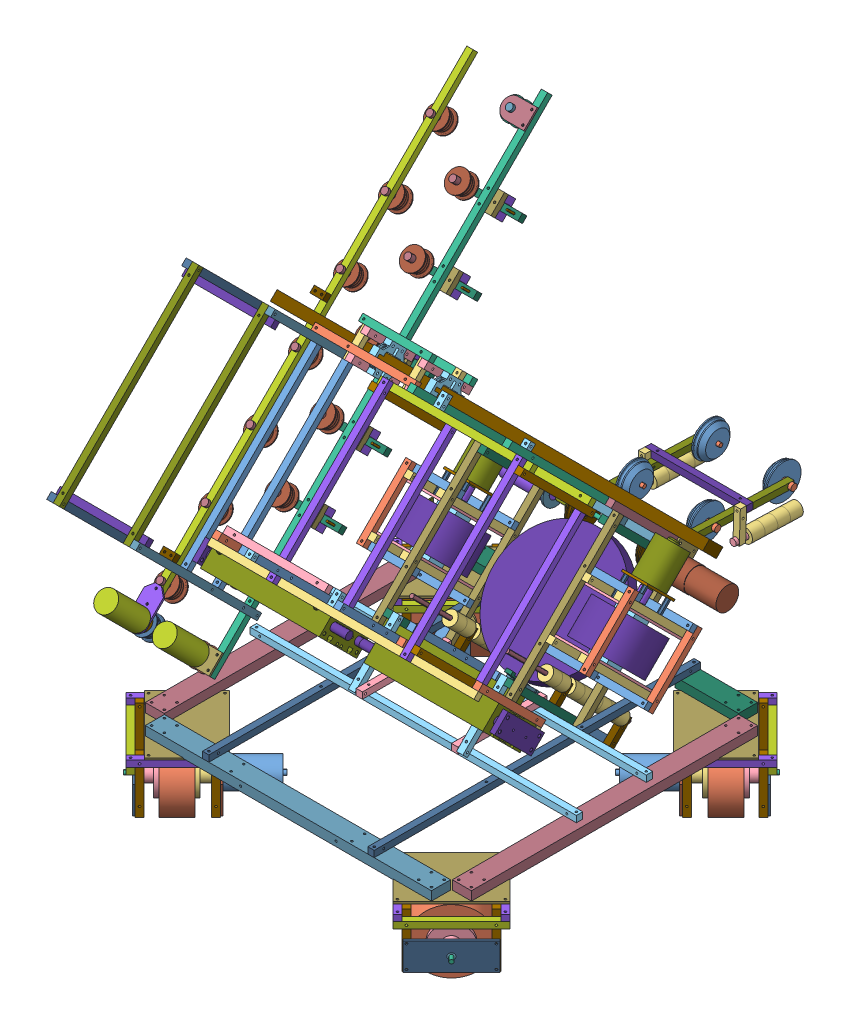
SolidWorks assembly R1, configuration ﾃﾞﾌｫﾙﾄ. Lengths in mm.
Overall size (700 795.51 1072.73).
351 component instances, 107 part files, 20 mates.
Components (placement in the parent):
- Copy of Runner^R1-1: Copy of Runner^R1 [ﾃﾞﾌｫﾙﾄ] at (-280.0303 -23.0504 467.0696) size (691.03 259.3 691.03) (virtual)
  - Copy of Copy of 足回り角^Copy of Runner_R1-1: Copy of Copy of 足回り角^Copy of Runner_R1 [ﾃﾞﾌｫﾙﾄ] at (-236.5804 -569.4039 -424.4309) x (0.322664 -0.429464 -0.843474) z (-0.833839 -0.550655 -0.038606) size (175.41 194.61 181.45) (virtual)
    - Copy of 足回りモータ^Copy of Copy of 足回り角_Copy of Runner_R1-1: Copy of 足回りモータ^Copy of Copy of 足回り角_Copy of Runner_R1 [ﾃﾞﾌｫﾙﾄ] at (-551.1259 26.8519 -574.9243) x (0.279393 -0.550081 -0.786989) z (0.886746 0.462184 -0.008244) size (42 98.4 42) (virtual)
    - Copy of 足回りE^Copy of Copy of 足回り角_Copy of Runner_R1-1: Copy of 足回りE^Copy of Copy of 足回り角_Copy of Runner_R1 [ﾃﾞﾌｫﾙﾄ] at (-524.7579 -22.9499 -530.7534) x (0.201013 -0.588283 -0.783273) z (0.907729 0.412462 -0.07683) size (100 40 100) (virtual)
    - Copy of Part11^Copy of Copy of 足回り角_Copy of Runner_R1-1: Copy of Part11^Copy of Copy of 足回り角_Copy of Runner_R1 [ﾃﾞﾌｫﾙﾄ] at (-688.5751 -7.1777 -584.6401) x (-0.368269 0.695555 -0.616912) z (-0.201013 0.588283 0.783273) size (26.4 56.8 56.8) (virtual)
    - Copy of Copy of Part11^Copy of Copy of 足回り角_Copy of Runner_R1-1: Copy of Copy of Part11^Copy of Copy of 足回り角_Copy of Runner_R1 [ﾃﾞﾌｫﾙﾄ] at (-522.8714 -163.2458 -585.4385) x (0.368269 -0.695555 0.616912) z (0.915702 0.156572 -0.370101) size (26.4 56.8 56.8) (virtual)
    - Part4^Copy of Copy of 足回り角_Copy of Runner_R1-7: Part4^Copy of Copy of 足回り角_Copy of Runner_R1 [ﾃﾞﾌｫﾙﾄ] at (-186.4359 394.8707 -734.6433) x (-0.368269 0.695555 -0.616912) z (0.907729 0.412462 -0.07683) size (2 10 10) (virtual)
    - Part5^Copy of Copy of 足回り角_Copy of Runner_R1-1: Part5^Copy of Copy of 足回り角_Copy of Runner_R1 [ﾃﾞﾌｫﾙﾄ] at (-68.1457 171.4539 -536.4872) x (0.907729 0.412462 -0.07683) z (0.368269 -0.695555 0.616912) size (6 6 35) (virtual)
    - Part6^Copy of Copy of 足回り角_Copy of Runner_R1-12: Part6^Copy of Copy of 足回り角_Copy of Runner_R1 [ﾃﾞﾌｫﾙﾄ] at (-467.3947 -89.0148 -566.7968) x (0.824584 -0.062152 -0.562315) z (-0.429464 -0.715779 -0.550655) size (130 10 10) (virtual)
    - Part6^Copy of Copy of 足回り角_Copy of Runner_R1-16: Part6^Copy of Copy of 足回り角_Copy of Runner_R1 [ﾃﾞﾌｫﾙﾄ] at (-520.2575 -4.441 -653.6633) x (0.824584 -0.062152 -0.562315) z (0.429464 0.715779 0.550655) size (130 10 10) (virtual)
    - Copy of Part6^Copy of Copy of 足回り角_Copy of Runner_R1-7: Copy of Part6^Copy of Copy of 足回り角_Copy of Runner_R1 [ﾃﾞﾌｫﾙﾄ] at (-544.6117 -11.2666 -643.957) x (-0.368269 0.695555 -0.616912) z (0.429464 0.715779 0.550655) size (115 10 10) (virtual)
    - Copy of Part6^Copy of Copy of 足回り角_Copy of Runner_R1-9: Copy of Part6^Copy of Copy of 足回り角_Copy of Runner_R1 [ﾃﾞﾌｫﾙﾄ] at (-643.5618 -3.8083 -576.4793) x (-0.368269 0.695555 -0.616912) z (0.429464 0.715779 0.550655) size (115 10 10) (virtual)
    - Copy of Copy of Part6^Copy of Copy of 足回り角_Copy of Runner_R1-1: Copy of Copy of Part6^Copy of Copy of 足回り角_Copy of Runner_R1 [ﾃﾞﾌｫﾙﾄ] at (-546.4038 -4.8062 -484.4742) x (0.429464 0.715779 0.550655) z (-0.824584 0.062152 0.562315) size (85 10 10) (virtual)
    - Copy of Copy of Part6^Copy of Copy of 足回り角_Copy of Runner_R1-2: Copy of Copy of Part6^Copy of Copy of 足回り角_Copy of Runner_R1 [ﾃﾞﾌｫﾙﾄ] at (-577.7066 54.316 -536.9118) x (0.429464 0.715779 0.550655) z (-0.824584 0.062152 0.562315) size (85 10 10) (virtual)
    - Copy of Copy of Part6^Copy of Copy of 足回り角_Copy of Runner_R1-3: Copy of Copy of Part6^Copy of Copy of 足回り角_Copy of Runner_R1 [ﾃﾞﾌｫﾙﾄ] at (-463.9454 -11.0215 -540.7057) x (0.429464 0.715779 0.550655) z (-0.824584 0.062152 0.562315) size (85 10 10) (virtual)
    - Copy of Copy of Part6^Copy of Copy of 足回り角_Copy of Runner_R1-4: Copy of Copy of Part6^Copy of Copy of 足回り角_Copy of Runner_R1 [ﾃﾞﾌｫﾙﾄ] at (-495.2482 48.1008 -593.1432) x (0.429464 0.715779 0.550655) z (-0.824584 0.062152 0.562315) size (85 10 10) (virtual)
    - Copy of Part7^Copy of Copy of 足回り角_Copy of Runner_R1-1: Copy of Part7^Copy of Copy of 足回り角_Copy of Runner_R1 [ﾃﾞﾌｫﾙﾄ] at (-536.2553 -8.1719 -459.5715) x (0.429464 0.715779 0.550655) z (-0.368269 0.695555 -0.616912) size (43 108 3) (virtual)
    - Part7^Copy of Copy of 足回り角_Copy of Runner_R1-3: Part7^Copy of Copy of 足回り角_Copy of Runner_R1 [ﾃﾞﾌｫﾙﾄ] at (-584.534 59.789 -512.9824) x (0.429464 0.715779 0.550655) z (-0.368269 0.695555 -0.616912) size (43 108 3) (virtual)
    - Part10^Copy of Copy of 足回り角_Copy of Runner_R1-2: Part10^Copy of Copy of 足回り角_Copy of Runner_R1 [ﾃﾞﾌｫﾙﾄ] at (-643.5618 -3.8083 -576.4793) x (0.368269 -0.695555 0.616912) z (-0.429464 -0.715779 -0.550655) size (94.7 130 3) (virtual)
  - Copy of Copy of 足回り角^Copy of Runner_R1-2: Copy of Copy of 足回り角^Copy of Runner_R1 [ﾃﾞﾌｫﾙﾄ] at (937.2593 -569.4039 -236.5804) x (0.843474 -0.429464 0.322664) z (0.038606 -0.550655 -0.833839) size (175.41 194.61 181.45) (virtual)
    - Copy of 足回りモータ^Copy of Copy of 足回り角_Copy of Runner_R1-1: Copy of 足回りモータ^Copy of Copy of 足回り角_Copy of Runner_R1 [ﾃﾞﾌｫﾙﾄ] at (-551.1259 26.8519 -574.9243) x (0.279393 -0.550081 -0.786989) z (0.886746 0.462184 -0.008244) size (42 98.4 42) (virtual)
    - Copy of 足回りE^Copy of Copy of 足回り角_Copy of Runner_R1-1: Copy of 足回りE^Copy of Copy of 足回り角_Copy of Runner_R1 [ﾃﾞﾌｫﾙﾄ] at (-524.7579 -22.9499 -530.7534) x (0.201013 -0.588283 -0.783273) z (0.907729 0.412462 -0.07683) size (100 40 100) (virtual)
    - Copy of Part11^Copy of Copy of 足回り角_Copy of Runner_R1-1: Copy of Part11^Copy of Copy of 足回り角_Copy of Runner_R1 [ﾃﾞﾌｫﾙﾄ] at (-688.5751 -7.1777 -584.6401) x (-0.368269 0.695555 -0.616912) z (-0.201013 0.588283 0.783273) size (26.4 56.8 56.8) (virtual)
    - Copy of Copy of Part11^Copy of Copy of 足回り角_Copy of Runner_R1-1: Copy of Copy of Part11^Copy of Copy of 足回り角_Copy of Runner_R1 [ﾃﾞﾌｫﾙﾄ] at (-522.8714 -163.2458 -585.4385) x (0.368269 -0.695555 0.616912) z (0.915702 0.156572 -0.370101) size (26.4 56.8 56.8) (virtual)
    - Part4^Copy of Copy of 足回り角_Copy of Runner_R1-7: Part4^Copy of Copy of 足回り角_Copy of Runner_R1 [ﾃﾞﾌｫﾙﾄ] at (-186.4359 394.8707 -734.6433) x (-0.368269 0.695555 -0.616912) z (0.907729 0.412462 -0.07683) size (2 10 10) (virtual)
    - Part5^Copy of Copy of 足回り角_Copy of Runner_R1-1: Part5^Copy of Copy of 足回り角_Copy of Runner_R1 [ﾃﾞﾌｫﾙﾄ] at (-68.1457 171.4539 -536.4872) x (0.907729 0.412462 -0.07683) z (0.368269 -0.695555 0.616912) size (6 6 35) (virtual)
    - Part6^Copy of Copy of 足回り角_Copy of Runner_R1-12: Part6^Copy of Copy of 足回り角_Copy of Runner_R1 [ﾃﾞﾌｫﾙﾄ] at (-467.3947 -89.0148 -566.7968) x (0.824584 -0.062152 -0.562315) z (-0.429464 -0.715779 -0.550655) size (130 10 10) (virtual)
    - Part6^Copy of Copy of 足回り角_Copy of Runner_R1-16: Part6^Copy of Copy of 足回り角_Copy of Runner_R1 [ﾃﾞﾌｫﾙﾄ] at (-520.2575 -4.441 -653.6633) x (0.824584 -0.062152 -0.562315) z (0.429464 0.715779 0.550655) size (130 10 10) (virtual)
    - Copy of Part6^Copy of Copy of 足回り角_Copy of Runner_R1-7: Copy of Part6^Copy of Copy of 足回り角_Copy of Runner_R1 [ﾃﾞﾌｫﾙﾄ] at (-544.6117 -11.2666 -643.957) x (-0.368269 0.695555 -0.616912) z (0.429464 0.715779 0.550655) size (115 10 10) (virtual)
    - Copy of Part6^Copy of Copy of 足回り角_Copy of Runner_R1-9: Copy of Part6^Copy of Copy of 足回り角_Copy of Runner_R1 [ﾃﾞﾌｫﾙﾄ] at (-643.5618 -3.8083 -576.4793) x (-0.368269 0.695555 -0.616912) z (0.429464 0.715779 0.550655) size (115 10 10) (virtual)
    - Copy of Copy of Part6^Copy of Copy of 足回り角_Copy of Runner_R1-1: Copy of Copy of Part6^Copy of Copy of 足回り角_Copy of Runner_R1 [ﾃﾞﾌｫﾙﾄ] at (-546.4038 -4.8062 -484.4742) x (0.429464 0.715779 0.550655) z (-0.824584 0.062152 0.562315) size (85 10 10) (virtual)
    - Copy of Copy of Part6^Copy of Copy of 足回り角_Copy of Runner_R1-2: Copy of Copy of Part6^Copy of Copy of 足回り角_Copy of Runner_R1 [ﾃﾞﾌｫﾙﾄ] at (-577.7066 54.316 -536.9118) x (0.429464 0.715779 0.550655) z (-0.824584 0.062152 0.562315) size (85 10 10) (virtual)
    - Copy of Copy of Part6^Copy of Copy of 足回り角_Copy of Runner_R1-3: Copy of Copy of Part6^Copy of Copy of 足回り角_Copy of Runner_R1 [ﾃﾞﾌｫﾙﾄ] at (-463.9454 -11.0215 -540.7057) x (0.429464 0.715779 0.550655) z (-0.824584 0.062152 0.562315) size (85 10 10) (virtual)
    - Copy of Copy of Part6^Copy of Copy of 足回り角_Copy of Runner_R1-4: Copy of Copy of Part6^Copy of Copy of 足回り角_Copy of Runner_R1 [ﾃﾞﾌｫﾙﾄ] at (-495.2482 48.1008 -593.1432) x (0.429464 0.715779 0.550655) z (-0.824584 0.062152 0.562315) size (85 10 10) (virtual)
    - Copy of Part7^Copy of Copy of 足回り角_Copy of Runner_R1-1: Copy of Part7^Copy of Copy of 足回り角_Copy of Runner_R1 [ﾃﾞﾌｫﾙﾄ] at (-536.2553 -8.1719 -459.5715) x (0.429464 0.715779 0.550655) z (-0.368269 0.695555 -0.616912) size (43 108 3) (virtual)
    - Part7^Copy of Copy of 足回り角_Copy of Runner_R1-3: Part7^Copy of Copy of 足回り角_Copy of Runner_R1 [ﾃﾞﾌｫﾙﾄ] at (-584.534 59.789 -512.9824) x (0.429464 0.715779 0.550655) z (-0.368269 0.695555 -0.616912) size (43 108 3) (virtual)
    - Part10^Copy of Copy of 足回り角_Copy of Runner_R1-2: Part10^Copy of Copy of 足回り角_Copy of Runner_R1 [ﾃﾞﾌｫﾙﾄ] at (-643.5618 -3.8083 -576.4793) x (0.368269 -0.695555 0.616912) z (-0.429464 -0.715779 -0.550655) size (94.7 130 3) (virtual)
  - Copy of Copy of 足回り角^Copy of Runner_R1-3: Copy of Copy of 足回り角^Copy of Runner_R1 [ﾃﾞﾌｫﾙﾄ] at (-424.4309 -569.4039 749.4088) x (-0.843474 -0.429464 -0.322664) z (-0.038606 -0.550655 0.833839) size (175.41 194.61 181.45) (virtual)
    - Copy of 足回りモータ^Copy of Copy of 足回り角_Copy of Runner_R1-1: Copy of 足回りモータ^Copy of Copy of 足回り角_Copy of Runner_R1 [ﾃﾞﾌｫﾙﾄ] at (-551.1259 26.8519 -574.9243) x (0.279393 -0.550081 -0.786989) z (0.886746 0.462184 -0.008244) size (42 98.4 42) (virtual)
    - Copy of 足回りE^Copy of Copy of 足回り角_Copy of Runner_R1-1: Copy of 足回りE^Copy of Copy of 足回り角_Copy of Runner_R1 [ﾃﾞﾌｫﾙﾄ] at (-524.7579 -22.9499 -530.7534) x (0.201013 -0.588283 -0.783273) z (0.907729 0.412462 -0.07683) size (100 40 100) (virtual)
    - Copy of Part11^Copy of Copy of 足回り角_Copy of Runner_R1-1: Copy of Part11^Copy of Copy of 足回り角_Copy of Runner_R1 [ﾃﾞﾌｫﾙﾄ] at (-688.5751 -7.1777 -584.6401) x (-0.368269 0.695555 -0.616912) z (-0.201013 0.588283 0.783273) size (26.4 56.8 56.8) (virtual)
    - Copy of Copy of Part11^Copy of Copy of 足回り角_Copy of Runner_R1-1: Copy of Copy of Part11^Copy of Copy of 足回り角_Copy of Runner_R1 [ﾃﾞﾌｫﾙﾄ] at (-522.8714 -163.2458 -585.4385) x (0.368269 -0.695555 0.616912) z (0.915702 0.156572 -0.370101) size (26.4 56.8 56.8) (virtual)
    - Part4^Copy of Copy of 足回り角_Copy of Runner_R1-7: Part4^Copy of Copy of 足回り角_Copy of Runner_R1 [ﾃﾞﾌｫﾙﾄ] at (-186.4359 394.8707 -734.6433) x (-0.368269 0.695555 -0.616912) z (0.907729 0.412462 -0.07683) size (2 10 10) (virtual)
    - Part5^Copy of Copy of 足回り角_Copy of Runner_R1-1: Part5^Copy of Copy of 足回り角_Copy of Runner_R1 [ﾃﾞﾌｫﾙﾄ] at (-68.1457 171.4539 -536.4872) x (0.907729 0.412462 -0.07683) z (0.368269 -0.695555 0.616912) size (6 6 35) (virtual)
    - Part6^Copy of Copy of 足回り角_Copy of Runner_R1-12: Part6^Copy of Copy of 足回り角_Copy of Runner_R1 [ﾃﾞﾌｫﾙﾄ] at (-467.3947 -89.0148 -566.7968) x (0.824584 -0.062152 -0.562315) z (-0.429464 -0.715779 -0.550655) size (130 10 10) (virtual)
    - Part6^Copy of Copy of 足回り角_Copy of Runner_R1-16: Part6^Copy of Copy of 足回り角_Copy of Runner_R1 [ﾃﾞﾌｫﾙﾄ] at (-520.2575 -4.441 -653.6633) x (0.824584 -0.062152 -0.562315) z (0.429464 0.715779 0.550655) size (130 10 10) (virtual)
    - Copy of Part6^Copy of Copy of 足回り角_Copy of Runner_R1-7: Copy of Part6^Copy of Copy of 足回り角_Copy of Runner_R1 [ﾃﾞﾌｫﾙﾄ] at (-544.6117 -11.2666 -643.957) x (-0.368269 0.695555 -0.616912) z (0.429464 0.715779 0.550655) size (115 10 10) (virtual)
    - Copy of Part6^Copy of Copy of 足回り角_Copy of Runner_R1-9: Copy of Part6^Copy of Copy of 足回り角_Copy of Runner_R1 [ﾃﾞﾌｫﾙﾄ] at (-643.5618 -3.8083 -576.4793) x (-0.368269 0.695555 -0.616912) z (0.429464 0.715779 0.550655) size (115 10 10) (virtual)
    - Copy of Copy of Part6^Copy of Copy of 足回り角_Copy of Runner_R1-1: Copy of Copy of Part6^Copy of Copy of 足回り角_Copy of Runner_R1 [ﾃﾞﾌｫﾙﾄ] at (-546.4038 -4.8062 -484.4742) x (0.429464 0.715779 0.550655) z (-0.824584 0.062152 0.562315) size (85 10 10) (virtual)
    - Copy of Copy of Part6^Copy of Copy of 足回り角_Copy of Runner_R1-2: Copy of Copy of Part6^Copy of Copy of 足回り角_Copy of Runner_R1 [ﾃﾞﾌｫﾙﾄ] at (-577.7066 54.316 -536.9118) x (0.429464 0.715779 0.550655) z (-0.824584 0.062152 0.562315) size (85 10 10) (virtual)
    - Copy of Copy of Part6^Copy of Copy of 足回り角_Copy of Runner_R1-3: Copy of Copy of Part6^Copy of Copy of 足回り角_Copy of Runner_R1 [ﾃﾞﾌｫﾙﾄ] at (-463.9454 -11.0215 -540.7057) x (0.429464 0.715779 0.550655) z (-0.824584 0.062152 0.562315) size (85 10 10) (virtual)
    - Copy of Copy of Part6^Copy of Copy of 足回り角_Copy of Runner_R1-4: Copy of Copy of Part6^Copy of Copy of 足回り角_Copy of Runner_R1 [ﾃﾞﾌｫﾙﾄ] at (-495.2482 48.1008 -593.1432) x (0.429464 0.715779 0.550655) z (-0.824584 0.062152 0.562315) size (85 10 10) (virtual)
    - Copy of Part7^Copy of Copy of 足回り角_Copy of Runner_R1-1: Copy of Part7^Copy of Copy of 足回り角_Copy of Runner_R1 [ﾃﾞﾌｫﾙﾄ] at (-536.2553 -8.1719 -459.5715) x (0.429464 0.715779 0.550655) z (-0.368269 0.695555 -0.616912) size (43 108 3) (virtual)
    - Part7^Copy of Copy of 足回り角_Copy of Runner_R1-3: Part7^Copy of Copy of 足回り角_Copy of Runner_R1 [ﾃﾞﾌｫﾙﾄ] at (-584.534 59.789 -512.9824) x (0.429464 0.715779 0.550655) z (-0.368269 0.695555 -0.616912) size (43 108 3) (virtual)
    - Part10^Copy of Copy of 足回り角_Copy of Runner_R1-2: Part10^Copy of Copy of 足回り角_Copy of Runner_R1 [ﾃﾞﾌｫﾙﾄ] at (-643.5618 -3.8083 -576.4793) x (0.368269 -0.695555 0.616912) z (-0.429464 -0.715779 -0.550655) size (94.7 130 3) (virtual)
  - Copy of Copy of 足回り角^Copy of Runner_R1-4: Copy of Copy of 足回り角^Copy of Runner_R1 [ﾃﾞﾌｫﾙﾄ] at (749.4088 -569.4039 937.2593) x (-0.322664 -0.429464 0.843474) z (0.833839 -0.550655 0.038606) size (175.41 194.61 181.45) (virtual)
    - Copy of 足回りモータ^Copy of Copy of 足回り角_Copy of Runner_R1-1: Copy of 足回りモータ^Copy of Copy of 足回り角_Copy of Runner_R1 [ﾃﾞﾌｫﾙﾄ] at (-551.1259 26.8519 -574.9243) x (0.279393 -0.550081 -0.786989) z (0.886746 0.462184 -0.008244) size (42 98.4 42) (virtual)
    - Copy of 足回りE^Copy of Copy of 足回り角_Copy of Runner_R1-1: Copy of 足回りE^Copy of Copy of 足回り角_Copy of Runner_R1 [ﾃﾞﾌｫﾙﾄ] at (-524.7579 -22.9499 -530.7534) x (0.201013 -0.588283 -0.783273) z (0.907729 0.412462 -0.07683) size (100 40 100) (virtual)
    - Copy of Part11^Copy of Copy of 足回り角_Copy of Runner_R1-1: Copy of Part11^Copy of Copy of 足回り角_Copy of Runner_R1 [ﾃﾞﾌｫﾙﾄ] at (-688.5751 -7.1777 -584.6401) x (-0.368269 0.695555 -0.616912) z (-0.201013 0.588283 0.783273) size (26.4 56.8 56.8) (virtual)
    - Copy of Copy of Part11^Copy of Copy of 足回り角_Copy of Runner_R1-1: Copy of Copy of Part11^Copy of Copy of 足回り角_Copy of Runner_R1 [ﾃﾞﾌｫﾙﾄ] at (-522.8714 -163.2458 -585.4385) x (0.368269 -0.695555 0.616912) z (0.915702 0.156572 -0.370101) size (26.4 56.8 56.8) (virtual)
    - Part4^Copy of Copy of 足回り角_Copy of Runner_R1-7: Part4^Copy of Copy of 足回り角_Copy of Runner_R1 [ﾃﾞﾌｫﾙﾄ] at (-186.4359 394.8707 -734.6433) x (-0.368269 0.695555 -0.616912) z (0.907729 0.412462 -0.07683) size (2 10 10) (virtual)
    - Part5^Copy of Copy of 足回り角_Copy of Runner_R1-1: Part5^Copy of Copy of 足回り角_Copy of Runner_R1 [ﾃﾞﾌｫﾙﾄ] at (-68.1457 171.4539 -536.4872) x (0.907729 0.412462 -0.07683) z (0.368269 -0.695555 0.616912) size (6 6 35) (virtual)
    - Part6^Copy of Copy of 足回り角_Copy of Runner_R1-12: Part6^Copy of Copy of 足回り角_Copy of Runner_R1 [ﾃﾞﾌｫﾙﾄ] at (-467.3947 -89.0148 -566.7968) x (0.824584 -0.062152 -0.562315) z (-0.429464 -0.715779 -0.550655) size (130 10 10) (virtual)
    - Part6^Copy of Copy of 足回り角_Copy of Runner_R1-16: Part6^Copy of Copy of 足回り角_Copy of Runner_R1 [ﾃﾞﾌｫﾙﾄ] at (-520.2575 -4.441 -653.6633) x (0.824584 -0.062152 -0.562315) z (0.429464 0.715779 0.550655) size (130 10 10) (virtual)
    - Copy of Part6^Copy of Copy of 足回り角_Copy of Runner_R1-7: Copy of Part6^Copy of Copy of 足回り角_Copy of Runner_R1 [ﾃﾞﾌｫﾙﾄ] at (-544.6117 -11.2666 -643.957) x (-0.368269 0.695555 -0.616912) z (0.429464 0.715779 0.550655) size (115 10 10) (virtual)
    - Copy of Part6^Copy of Copy of 足回り角_Copy of Runner_R1-9: Copy of Part6^Copy of Copy of 足回り角_Copy of Runner_R1 [ﾃﾞﾌｫﾙﾄ] at (-643.5618 -3.8083 -576.4793) x (-0.368269 0.695555 -0.616912) z (0.429464 0.715779 0.550655) size (115 10 10) (virtual)
    - Copy of Copy of Part6^Copy of Copy of 足回り角_Copy of Runner_R1-1: Copy of Copy of Part6^Copy of Copy of 足回り角_Copy of Runner_R1 [ﾃﾞﾌｫﾙﾄ] at (-546.4038 -4.8062 -484.4742) x (0.429464 0.715779 0.550655) z (-0.824584 0.062152 0.562315) size (85 10 10) (virtual)
    - Copy of Copy of Part6^Copy of Copy of 足回り角_Copy of Runner_R1-2: Copy of Copy of Part6^Copy of Copy of 足回り角_Copy of Runner_R1 [ﾃﾞﾌｫﾙﾄ] at (-577.7066 54.316 -536.9118) x (0.429464 0.715779 0.550655) z (-0.824584 0.062152 0.562315) size (85 10 10) (virtual)
    - Copy of Copy of Part6^Copy of Copy of 足回り角_Copy of Runner_R1-3: Copy of Copy of Part6^Copy of Copy of 足回り角_Copy of Runner_R1 [ﾃﾞﾌｫﾙﾄ] at (-463.9454 -11.0215 -540.7057) x (0.429464 0.715779 0.550655) z (-0.824584 0.062152 0.562315) size (85 10 10) (virtual)
    - Copy of Copy of Part6^Copy of Copy of 足回り角_Copy of Runner_R1-4: Copy of Copy of Part6^Copy of Copy of 足回り角_Copy of Runner_R1 [ﾃﾞﾌｫﾙﾄ] at (-495.2482 48.1008 -593.1432) x (0.429464 0.715779 0.550655) z (-0.824584 0.062152 0.562315) size (85 10 10) (virtual)
    - Copy of Part7^Copy of Copy of 足回り角_Copy of Runner_R1-1: Copy of Part7^Copy of Copy of 足回り角_Copy of Runner_R1 [ﾃﾞﾌｫﾙﾄ] at (-536.2553 -8.1719 -459.5715) x (0.429464 0.715779 0.550655) z (-0.368269 0.695555 -0.616912) size (43 108 3) (virtual)
    - Part7^Copy of Copy of 足回り角_Copy of Runner_R1-3: Part7^Copy of Copy of 足回り角_Copy of Runner_R1 [ﾃﾞﾌｫﾙﾄ] at (-584.534 59.789 -512.9824) x (0.429464 0.715779 0.550655) z (-0.368269 0.695555 -0.616912) size (43 108 3) (virtual)
    - Part10^Copy of Copy of 足回り角_Copy of Runner_R1-2: Part10^Copy of Copy of 足回り角_Copy of Runner_R1 [ﾃﾞﾌｫﾙﾄ] at (-643.5618 -3.8083 -576.4793) x (0.368269 -0.695555 0.616912) z (-0.429464 -0.715779 -0.550655) size (94.7 130 3) (virtual)
  - Part9^Copy of Runner_R1-1: Part9^Copy of Runner_R1 [ﾃﾞﾌｫﾙﾄ] at (521.6964 29.1498 330.8565) x (0 0 -1) z (0 1 0) size (450 30 15) (virtual)
  - Copy of Part9^Copy of Runner_R1-1: Copy of Part9^Copy of Runner_R1 [ﾃﾞﾌｫﾙﾄ] at (330.3437 44.1498 521.6964) x (-1 0 0) z (0 -1 0) size (450 30 15) (virtual)
  - Part9^Copy of Runner_R1-3: Part9^Copy of Runner_R1 [ﾃﾞﾌｫﾙﾄ] at (-8.868 29.1498 181.972) x (0 0 1) z (0 1 0) size (450 30 15) (virtual)
  - Copy (2) of Part9^Copy of Runner_R1-1: Copy (2) of Part9^Copy of Runner_R1 [ﾃﾞﾌｫﾙﾄ] at (-19.1435 29.1498 -8.868) x (-1 0 0) z (0 1 0) size (100 30 15) (virtual)
  - Copy (2) of Part9^Copy of Runner_R1-2: Copy (2) of Part9^Copy of Runner_R1 [ﾃﾞﾌｫﾙﾄ] at (531.972 29.1498 38.868) x (1 0 0) z (0 1 0) size (100 30 15) (virtual)
- Copy of Shooter^R1-1: Copy of Shooter^R1 [ﾃﾞﾌｫﾙﾄ] at (-133.6161 -3.3981 632.9203) x (1 0 0) z (0 0.707107 0.707107) size (512.8 479.46 353.57) (virtual, flexible)
  - Copy of Roller^Copy of Shooter_R1-1: Copy of Roller^Copy of Shooter_R1 [ﾃﾞﾌｫﾙﾄ] at (-59.3841 78.5441 92.0532) x (0.999685 0 0.025079) z (-0.025079 0 0.999685) size (101.44 180.8 151.71) (virtual)
    - Copy of Copy of motor^Copy of Roller_Copy of Shooter_R1-1: Copy of Copy of motor^Copy of Roller_Copy of Shooter_R1 [ﾃﾞﾌｫﾙﾄ] at (28.9472 162.9559 -17.7848) x (0.025079 0 0.999685) z (0 -1 0) size (45 45 69.7) (virtual)
    - Copy of Roller^Copy of Roller_Copy of Shooter_R1-1: Copy of Roller^Copy of Roller_Copy of Shooter_R1 [ﾃﾞﾌｫﾙﾄ] at (28.9472 14.4559 -17.7848) x (0.999895 0 0.0145) z (-0.0145 0 0.999895) size (100 54 100) (virtual)
    - Part6^Copy of Roller_Copy of Shooter_R1-1: Part6^Copy of Roller_Copy of Shooter_R1 [ﾃﾞﾌｫﾙﾄ] at (28.9472 29.4559 -17.7848) x (-0.999895 0 -0.0145) z (-0.0145 0 0.999895) size (28 15 28) (virtual)
    - Copy of Copy (2) of Copy of Copy (2) of 角材１^Copy of Roller_Copy of Shooter_R1-1: Copy of Copy (2) of Copy of Copy (2) of 角材１^Copy of Roller_Copy of Shooter_R1 [ﾃﾞﾌｫﾙﾄ] at (-9.6609 -13.5441 38.2011) x (0.999685 0 -0.025079) z (0.025079 0 0.999685) size (80 10 10) (virtual)
    - Copy of Copy (2) of Copy of Copy (2) of 角材１^Copy of Roller_Copy of Shooter_R1-2: Copy of Copy (2) of Copy of Copy (2) of 角材１^Copy of Roller_Copy of Shooter_R1 [ﾃﾞﾌｫﾙﾄ] at (-12.6704 -13.5441 -81.7612) x (0.999685 0 -0.025079) z (0.025079 0 0.999685) size (80 10 10) (virtual)
    - Copy of Copy of Copy (2) of Copy of Copy (2) of 角材１^Copy of Roller_Copy of Shooter_R1-2: Copy of Copy of Copy (2) of Copy of Copy (2) of 角材１^Copy of Roller_Copy of Shooter_R1 [ﾃﾞﾌｫﾙﾄ] at (-9.4101 96.4559 48.1979) x (0 -1 0) z (0.025079 0 0.999685) size (110 10 10) (virtual)
    - Copy of Copy of Copy (2) of Copy of Copy (2) of 角材１^Copy of Roller_Copy of Shooter_R1-4: Copy of Copy of Copy (2) of Copy of Copy (2) of 角材１^Copy of Roller_Copy of Shooter_R1 [ﾃﾞﾌｫﾙﾄ] at (-12.9212 96.4559 -91.7581) x (0 -1 0) z (0.025079 0 0.999685) size (110 10 10) (virtual)
    - Copy (2) of Copy of Copy (2) of Copy of Copy (2) of 角材１^Copy of Roller_Copy of Shooter_R1-1: Copy (2) of Copy of Copy (2) of Copy of Copy (2) of 角材１^Copy of Roller_Copy of Shooter_R1 [ﾃﾞﾌｫﾙﾄ] at (57.0568 -3.5441 -93.5136) x (0.025079 0 0.999685) z (-0.999685 0 0.025079) size (150 10 10) (virtual)
    - Copy (2) of Copy of Copy (2) of Copy of Copy (2) of 角材１^Copy of Roller_Copy of Shooter_R1-2: Copy (2) of Copy of Copy (2) of Copy of Copy (2) of 角材１^Copy of Roller_Copy of Shooter_R1 [ﾃﾞﾌｫﾙﾄ] at (7.0725 -3.5441 -92.2596) x (0.025079 0 0.999685) z (-0.999685 0 0.025079) size (150 10 10) (virtual)
    - Copy (2) of Copy of Copy (2) of Copy of Copy (2) of 角材１^Copy of Roller_Copy of Shooter_R1-3: Copy (2) of Copy of Copy (2) of Copy of Copy (2) of 角材１^Copy of Roller_Copy of Shooter_R1 [ﾃﾞﾌｫﾙﾄ] at (7.0725 76.4559 -92.2596) x (0.025079 0 0.999685) z (-0.999685 0 0.025079) size (150 10 10) (virtual)
    - Copy (2) of Copy of Copy (2) of Copy of Copy (2) of 角材１^Copy of Roller_Copy of Shooter_R1-4: Copy (2) of Copy of Copy (2) of Copy of Copy (2) of 角材１^Copy of Roller_Copy of Shooter_R1 [ﾃﾞﾌｫﾙﾄ] at (57.0568 76.4559 -93.5136) x (0.025079 0 0.999685) z (-0.999685 0 0.025079) size (150 10 10) (virtual)
    - Copy of Copy (2) of Copy of Copy (2) of 角材１^Copy of Roller_Copy of Shooter_R1-5: Copy of Copy (2) of Copy of Copy (2) of 角材１^Copy of Roller_Copy of Shooter_R1 [ﾃﾞﾌｫﾙﾄ] at (-12.6704 86.4559 -81.7612) x (0.999685 0 -0.025079) z (0.025079 0 0.999685) size (80 10 10) (virtual)
    - Copy of Copy (2) of Copy of Copy (2) of 角材１^Copy of Roller_Copy of Shooter_R1-6: Copy of Copy (2) of Copy of Copy (2) of 角材１^Copy of Roller_Copy of Shooter_R1 [ﾃﾞﾌｫﾙﾄ] at (-9.6609 86.4559 38.2011) x (0.999685 0 -0.025079) z (0.025079 0 0.999685) size (80 10 10) (virtual)
    - Part8^Copy of Roller_Copy of Shooter_R1-1: Part8^Copy of Roller_Copy of Shooter_R1 [ﾃﾞﾌｫﾙﾄ] at (-2.6735 6.4559 -82.012) x (0.025079 0 0.999685) z (0 1 0) size (130 60 3) (virtual)
    - Part9^Copy of Roller_Copy of Shooter_R1-1: Part9^Copy of Roller_Copy of Shooter_R1 [ﾃﾞﾌｫﾙﾄ] at (13.5757 9.4559 -32.4039) x (0.025079 0 0.999685) z (0 1 0) size (30 30 5) (virtual)
    - Part8^Copy of Roller_Copy of Shooter_R1-2: Part8^Copy of Roller_Copy of Shooter_R1 [ﾃﾞﾌｫﾙﾄ] at (57.3076 76.4559 -83.5168) x (0.025079 0 0.999685) z (0 -1 0) size (130 60 3) (virtual)
    - Part9^Copy of Roller_Copy of Shooter_R1-2: Part9^Copy of Roller_Copy of Shooter_R1 [ﾃﾞﾌｫﾙﾄ] at (43.5663 73.4559 -33.1563) x (0.025079 0 0.999685) z (0 -1 0) size (30 30 5) (virtual)
    - Part10^Copy of Roller_Copy of Shooter_R1-1: Part10^Copy of Roller_Copy of Shooter_R1 [ﾃﾞﾌｫﾙﾄ] at (43.5663 68.4559 -33.1563) x (0.025079 0 0.999685) z (0 -1 0) size (30 30 2) (virtual)
    - Part10^Copy of Roller_Copy of Shooter_R1-2: Part10^Copy of Roller_Copy of Shooter_R1 [ﾃﾞﾌｫﾙﾄ] at (43.5663 16.4559 -33.1563) x (0.025079 0 0.999685) z (0 -1 0) size (30 30 2) (virtual)
    - Part6^Copy of Roller_Copy of Shooter_R1-2: Part6^Copy of Roller_Copy of Shooter_R1 [ﾃﾞﾌｫﾙﾄ] at (28.9472 37.4559 -17.7848) x (0.999895 0 0.0145) z (-0.0145 0 0.999895) size (28 15 28) (virtual)
    - Part11^Copy of Roller_Copy of Shooter_R1-1: Part11^Copy of Roller_Copy of Shooter_R1 [ﾃﾞﾌｫﾙﾄ] at (28.9472 -2.4441 -17.7848) x (0 1 0) z (-0.999993 0 0.003776) size (100 6 6) (virtual)
    - Part12^Copy of Roller_Copy of Shooter_R1-1: Part12^Copy of Roller_Copy of Shooter_R1 [ﾃﾞﾌｫﾙﾄ] at (28.9472 87.0559 -17.7848) x (0.99763 0 -0.068811) z (0 1 0) size (16 16 18) (virtual)
    - Part13^Copy of Roller_Copy of Shooter_R1-1: Part13^Copy of Roller_Copy of Shooter_R1 [ﾃﾞﾌｫﾙﾄ] at (28.9472 109.4559 -17.7848) x (-0.999685 0 0.025079) z (0 -1 0) size (40 60 3) (virtual)
    - Part14^Copy of Roller_Copy of Shooter_R1-1: Part14^Copy of Roller_Copy of Shooter_R1 [ﾃﾞﾌｫﾙﾄ] at (14.5789 76.4559 7.5835) x (-0.003776 0 -0.999993) z (0 1 0) size (6.34 5.64 30) (virtual)
    - Part14^Copy of Roller_Copy of Shooter_R1-2: Part14^Copy of Roller_Copy of Shooter_R1 [ﾃﾞﾌｫﾙﾄ] at (43.3155 76.4559 -43.1531) x (-0.003776 0 -0.999993) z (0 1 0) size (6.34 5.64 30) (virtual)
    - Part14^Copy of Roller_Copy of Shooter_R1-3: Part14^Copy of Roller_Copy of Shooter_R1 [ﾃﾞﾌｫﾙﾄ] at (44.5695 76.4559 6.8311) x (-0.003776 0 -0.999993) z (0 1 0) size (6.34 5.64 30) (virtual)
    - Part14^Copy of Roller_Copy of Shooter_R1-4: Part14^Copy of Roller_Copy of Shooter_R1 [ﾃﾞﾌｫﾙﾄ] at (13.3249 76.4559 -42.4008) x (-0.003776 0 -0.999993) z (0 1 0) size (6.34 5.64 30) (virtual)
    - Part15^Copy of Roller_Copy of Shooter_R1-1: Part15^Copy of Roller_Copy of Shooter_R1 [ﾃﾞﾌｫﾙﾄ] at (28.9472 14.4559 -17.7848) x (0.00379 0 0.999993) z (0 -1 0) size (13 13 5) (virtual)
    - Part15^Copy of Roller_Copy of Shooter_R1-2: Part15^Copy of Roller_Copy of Shooter_R1 [ﾃﾞﾌｫﾙﾄ] at (28.9472 73.4559 -17.7848) x (0.00379 0 0.999993) z (0 -1 0) size (13 13 5) (virtual)
  - Copy of Roller^Copy of Shooter_R1-2: Copy of Roller^Copy of Shooter_R1 [ﾃﾞﾌｫﾙﾄ] at (279.3841 78.5441 57.9468) x (-0.999685 0 -0.025079) z (0.025079 0 -0.999685) size (101.44 180.8 151.71) (virtual)
    - Copy of Copy of motor^Copy of Roller_Copy of Shooter_R1-1: Copy of Copy of motor^Copy of Roller_Copy of Shooter_R1 [ﾃﾞﾌｫﾙﾄ] at (28.9472 162.9559 -17.7848) x (0.025079 0 0.999685) z (0 -1 0) size (45 45 69.7) (virtual)
    - Copy of Roller^Copy of Roller_Copy of Shooter_R1-1: Copy of Roller^Copy of Roller_Copy of Shooter_R1 [ﾃﾞﾌｫﾙﾄ] at (28.9472 14.4559 -17.7848) x (0.999895 0 0.0145) z (-0.0145 0 0.999895) size (100 54 100) (virtual)
    - Part6^Copy of Roller_Copy of Shooter_R1-1: Part6^Copy of Roller_Copy of Shooter_R1 [ﾃﾞﾌｫﾙﾄ] at (28.9472 29.4559 -17.7848) x (-0.999895 0 -0.0145) z (-0.0145 0 0.999895) size (28 15 28) (virtual)
    - Copy of Copy (2) of Copy of Copy (2) of 角材１^Copy of Roller_Copy of Shooter_R1-1: Copy of Copy (2) of Copy of Copy (2) of 角材１^Copy of Roller_Copy of Shooter_R1 [ﾃﾞﾌｫﾙﾄ] at (-9.6609 -13.5441 38.2011) x (0.999685 0 -0.025079) z (0.025079 0 0.999685) size (80 10 10) (virtual)
    - Copy of Copy (2) of Copy of Copy (2) of 角材１^Copy of Roller_Copy of Shooter_R1-2: Copy of Copy (2) of Copy of Copy (2) of 角材１^Copy of Roller_Copy of Shooter_R1 [ﾃﾞﾌｫﾙﾄ] at (-12.6704 -13.5441 -81.7612) x (0.999685 0 -0.025079) z (0.025079 0 0.999685) size (80 10 10) (virtual)
    - Copy of Copy of Copy (2) of Copy of Copy (2) of 角材１^Copy of Roller_Copy of Shooter_R1-2: Copy of Copy of Copy (2) of Copy of Copy (2) of 角材１^Copy of Roller_Copy of Shooter_R1 [ﾃﾞﾌｫﾙﾄ] at (-9.4101 96.4559 48.1979) x (0 -1 0) z (0.025079 0 0.999685) size (110 10 10) (virtual)
    - Copy of Copy of Copy (2) of Copy of Copy (2) of 角材１^Copy of Roller_Copy of Shooter_R1-4: Copy of Copy of Copy (2) of Copy of Copy (2) of 角材１^Copy of Roller_Copy of Shooter_R1 [ﾃﾞﾌｫﾙﾄ] at (-12.9212 96.4559 -91.7581) x (0 -1 0) z (0.025079 0 0.999685) size (110 10 10) (virtual)
    - Copy (2) of Copy of Copy (2) of Copy of Copy (2) of 角材１^Copy of Roller_Copy of Shooter_R1-1: Copy (2) of Copy of Copy (2) of Copy of Copy (2) of 角材１^Copy of Roller_Copy of Shooter_R1 [ﾃﾞﾌｫﾙﾄ] at (57.0568 -3.5441 -93.5136) x (0.025079 0 0.999685) z (-0.999685 0 0.025079) size (150 10 10) (virtual)
    - Copy (2) of Copy of Copy (2) of Copy of Copy (2) of 角材１^Copy of Roller_Copy of Shooter_R1-2: Copy (2) of Copy of Copy (2) of Copy of Copy (2) of 角材１^Copy of Roller_Copy of Shooter_R1 [ﾃﾞﾌｫﾙﾄ] at (7.0725 -3.5441 -92.2596) x (0.025079 0 0.999685) z (-0.999685 0 0.025079) size (150 10 10) (virtual)
    - Copy (2) of Copy of Copy (2) of Copy of Copy (2) of 角材１^Copy of Roller_Copy of Shooter_R1-3: Copy (2) of Copy of Copy (2) of Copy of Copy (2) of 角材１^Copy of Roller_Copy of Shooter_R1 [ﾃﾞﾌｫﾙﾄ] at (7.0725 76.4559 -92.2596) x (0.025079 0 0.999685) z (-0.999685 0 0.025079) size (150 10 10) (virtual)
    - Copy (2) of Copy of Copy (2) of Copy of Copy (2) of 角材１^Copy of Roller_Copy of Shooter_R1-4: Copy (2) of Copy of Copy (2) of Copy of Copy (2) of 角材１^Copy of Roller_Copy of Shooter_R1 [ﾃﾞﾌｫﾙﾄ] at (57.0568 76.4559 -93.5136) x (0.025079 0 0.999685) z (-0.999685 0 0.025079) size (150 10 10) (virtual)
    - Copy of Copy (2) of Copy of Copy (2) of 角材１^Copy of Roller_Copy of Shooter_R1-5: Copy of Copy (2) of Copy of Copy (2) of 角材１^Copy of Roller_Copy of Shooter_R1 [ﾃﾞﾌｫﾙﾄ] at (-12.6704 86.4559 -81.7612) x (0.999685 0 -0.025079) z (0.025079 0 0.999685) size (80 10 10) (virtual)
    - Copy of Copy (2) of Copy of Copy (2) of 角材１^Copy of Roller_Copy of Shooter_R1-6: Copy of Copy (2) of Copy of Copy (2) of 角材１^Copy of Roller_Copy of Shooter_R1 [ﾃﾞﾌｫﾙﾄ] at (-9.6609 86.4559 38.2011) x (0.999685 0 -0.025079) z (0.025079 0 0.999685) size (80 10 10) (virtual)
    - Part8^Copy of Roller_Copy of Shooter_R1-1: Part8^Copy of Roller_Copy of Shooter_R1 [ﾃﾞﾌｫﾙﾄ] at (-2.6735 6.4559 -82.012) x (0.025079 0 0.999685) z (0 1 0) size (130 60 3) (virtual)
    - Part9^Copy of Roller_Copy of Shooter_R1-1: Part9^Copy of Roller_Copy of Shooter_R1 [ﾃﾞﾌｫﾙﾄ] at (13.5757 9.4559 -32.4039) x (0.025079 0 0.999685) z (0 1 0) size (30 30 5) (virtual)
    - Part8^Copy of Roller_Copy of Shooter_R1-2: Part8^Copy of Roller_Copy of Shooter_R1 [ﾃﾞﾌｫﾙﾄ] at (57.3076 76.4559 -83.5168) x (0.025079 0 0.999685) z (0 -1 0) size (130 60 3) (virtual)
    - Part9^Copy of Roller_Copy of Shooter_R1-2: Part9^Copy of Roller_Copy of Shooter_R1 [ﾃﾞﾌｫﾙﾄ] at (43.5663 73.4559 -33.1563) x (0.025079 0 0.999685) z (0 -1 0) size (30 30 5) (virtual)
    - Part10^Copy of Roller_Copy of Shooter_R1-1: Part10^Copy of Roller_Copy of Shooter_R1 [ﾃﾞﾌｫﾙﾄ] at (43.5663 68.4559 -33.1563) x (0.025079 0 0.999685) z (0 -1 0) size (30 30 2) (virtual)
    - Part10^Copy of Roller_Copy of Shooter_R1-2: Part10^Copy of Roller_Copy of Shooter_R1 [ﾃﾞﾌｫﾙﾄ] at (43.5663 16.4559 -33.1563) x (0.025079 0 0.999685) z (0 -1 0) size (30 30 2) (virtual)
    - Part6^Copy of Roller_Copy of Shooter_R1-2: Part6^Copy of Roller_Copy of Shooter_R1 [ﾃﾞﾌｫﾙﾄ] at (28.9472 37.4559 -17.7848) x (0.999895 0 0.0145) z (-0.0145 0 0.999895) size (28 15 28) (virtual)
    - Part11^Copy of Roller_Copy of Shooter_R1-1: Part11^Copy of Roller_Copy of Shooter_R1 [ﾃﾞﾌｫﾙﾄ] at (28.9472 -2.4441 -17.7848) x (0 1 0) z (-0.999993 0 0.003776) size (100 6 6) (virtual)
    - Part12^Copy of Roller_Copy of Shooter_R1-1: Part12^Copy of Roller_Copy of Shooter_R1 [ﾃﾞﾌｫﾙﾄ] at (28.9472 87.0559 -17.7848) x (0.99763 0 -0.068811) z (0 1 0) size (16 16 18) (virtual)
    - Part13^Copy of Roller_Copy of Shooter_R1-1: Part13^Copy of Roller_Copy of Shooter_R1 [ﾃﾞﾌｫﾙﾄ] at (28.9472 109.4559 -17.7848) x (-0.999685 0 0.025079) z (0 -1 0) size (40 60 3) (virtual)
    - Part14^Copy of Roller_Copy of Shooter_R1-1: Part14^Copy of Roller_Copy of Shooter_R1 [ﾃﾞﾌｫﾙﾄ] at (14.5789 76.4559 7.5835) x (-0.003776 0 -0.999993) z (0 1 0) size (6.34 5.64 30) (virtual)
    - Part14^Copy of Roller_Copy of Shooter_R1-2: Part14^Copy of Roller_Copy of Shooter_R1 [ﾃﾞﾌｫﾙﾄ] at (43.3155 76.4559 -43.1531) x (-0.003776 0 -0.999993) z (0 1 0) size (6.34 5.64 30) (virtual)
    - Part14^Copy of Roller_Copy of Shooter_R1-3: Part14^Copy of Roller_Copy of Shooter_R1 [ﾃﾞﾌｫﾙﾄ] at (44.5695 76.4559 6.8311) x (-0.003776 0 -0.999993) z (0 1 0) size (6.34 5.64 30) (virtual)
    - Part14^Copy of Roller_Copy of Shooter_R1-4: Part14^Copy of Roller_Copy of Shooter_R1 [ﾃﾞﾌｫﾙﾄ] at (13.3249 76.4559 -42.4008) x (-0.003776 0 -0.999993) z (0 1 0) size (6.34 5.64 30) (virtual)
    - Part15^Copy of Roller_Copy of Shooter_R1-1: Part15^Copy of Roller_Copy of Shooter_R1 [ﾃﾞﾌｫﾙﾄ] at (28.9472 14.4559 -17.7848) x (0.00379 0 0.999993) z (0 -1 0) size (13 13 5) (virtual)
    - Part15^Copy of Roller_Copy of Shooter_R1-2: Part15^Copy of Roller_Copy of Shooter_R1 [ﾃﾞﾌｫﾙﾄ] at (28.9472 73.4559 -17.7848) x (0.00379 0 0.999993) z (0 -1 0) size (13 13 5) (virtual)
  - Copy of Copy of Copy of Copy of Copy of Copy (2) of Copy of Copy (2) of 角材１^Copy of Shooter_R1-1: Copy of Copy of Copy of Copy of Copy of Copy (2) of Copy of Copy (2) of 角材１^Copy of Shooter_R1 [ﾃﾞﾌｫﾙﾄ] at (0 240 140) x (0 -1 0) z (0 0 1) size (240 10 10) (virtual)
  - Part17^Copy of Shooter_R1-1: Part17^Copy of Shooter_R1 [ﾃﾞﾌｫﾙﾄ] at (185 45 -115) x (0.916853 -0.399226 0) z (0 0 1) size (6 6 270) (virtual)
  - Copy of Copy of Copy of Copy of Copy of Copy (2) of Copy of Copy (2) of 角材１^Copy of Shooter_R1-2: Copy of Copy of Copy of Copy of Copy of Copy (2) of Copy of Copy (2) of 角材１^Copy of Shooter_R1 [ﾃﾞﾌｫﾙﾄ] at (0 240 0) x (0 -1 0) z (0 0 1) size (240 10 10) (virtual)
  - Copy of Copy of Copy of Copy of Copy (2) of Copy of Copy (2) of 角材１^Copy of Shooter_R1-2: Copy of Copy of Copy of Copy of Copy (2) of Copy of Copy (2) of 角材１^Copy of Shooter_R1 [ﾃﾞﾌｫﾙﾄ] at (0 230 10) size (220 10 10) (virtual)
  - Copy of Copy of Copy of Copy of Copy (2) of Copy of Copy (2) of 角材１^Copy of Shooter_R1-5: Copy of Copy of Copy of Copy of Copy (2) of Copy of Copy (2) of 角材１^Copy of Shooter_R1 [ﾃﾞﾌｫﾙﾄ] at (0 230 130) size (220 10 10) (virtual)
  - Copy of Copy of Copy (2) of Copy of Copy (2) of Copy of Copy (2) of 角材１^Copy of Shooter_R1-1: Copy of Copy of Copy (2) of Copy of Copy (2) of Copy of Copy (2) of 角材１^Copy of Shooter_R1 [ﾃﾞﾌｫﾙﾄ] at (20 220 0) x (0 0 1) z (-1 0 0) size (150 10 10) (virtual)
  - Copy of Copy of Copy (2) of Copy of Copy (2) of Copy of Copy (2) of 角材１^Copy of Shooter_R1-2: Copy of Copy of Copy (2) of Copy of Copy (2) of Copy of Copy (2) of 角材１^Copy of Shooter_R1 [ﾃﾞﾌｫﾙﾄ] at (210 220 0) x (0 0 1) z (-1 0 0) size (150 10 10) (virtual)
  - Copy of Copy of Copy of Copy of Copy of Copy (2) of Copy of Copy (2) of 角材１^Copy of Shooter_R1-3: Copy of Copy of Copy of Copy of Copy of Copy (2) of Copy of Copy (2) of 角材１^Copy of Shooter_R1 [ﾃﾞﾌｫﾙﾄ] at (210 240 140) x (0 -1 0) z (0 0 1) size (240 10 10) (virtual)
  - Copy of Copy of Copy of Copy of Copy of Copy (2) of Copy of Copy (2) of 角材１^Copy of Shooter_R1-4: Copy of Copy of Copy of Copy of Copy of Copy (2) of Copy of Copy (2) of 角材１^Copy of Shooter_R1 [ﾃﾞﾌｫﾙﾄ] at (210 240 0) x (0 -1 0) z (0 0 1) size (240 10 10) (virtual)
  - Copy of Copy (4) of Copy of Copy of Copy of Copy of Copy (2) of Copy of Copy (2) of 角材１^Copy of Shooter_R1-1: Copy of Copy (4) of Copy of Copy of Copy of Copy of Copy (2) of Copy of Copy (2) of 角材１^Copy of Shooter_R1 [ﾃﾞﾌｫﾙﾄ] at (0 0 130) size (220 10 10) (virtual)
  - Copy of Copy of Copy (2) of Copy of Copy (2) of Copy of Copy (2) of 角材１^Copy of Shooter_R1-3: Copy of Copy of Copy (2) of Copy of Copy (2) of Copy of Copy (2) of 角材１^Copy of Shooter_R1 [ﾃﾞﾌｫﾙﾄ] at (20 10 0) x (0 0 1) z (-1 0 0) size (150 10 10) (virtual)
  - Copy of Copy of Copy (2) of Copy of Copy (2) of Copy of Copy (2) of 角材１^Copy of Shooter_R1-4: Copy of Copy of Copy (2) of Copy of Copy (2) of Copy of Copy (2) of 角材１^Copy of Shooter_R1 [ﾃﾞﾌｫﾙﾄ] at (210 10 0) x (0 0 1) z (-1 0 0) size (150 10 10) (virtual)
  - Part19^Copy of Shooter_R1-1: Part19^Copy of Shooter_R1 [ﾃﾞﾌｫﾙﾄ] at (290 165 10) x (-1 0 0) z (0 0 -1) size (190 190 20) (virtual)
  - Copy (2) of Copy of Copy of Copy of Copy of Copy (2) of Copy of Copy (2) of 角材１^Copy of Shooter_R1-3: Copy (2) of Copy of Copy of Copy of Copy of Copy (2) of Copy of Copy (2) of 角材１^Copy of Shooter_R1 [ﾃﾞﾌｫﾙﾄ] at (180 50 20) x (0 -1 0) z (0 0 1) size (50 10 10) (virtual)
